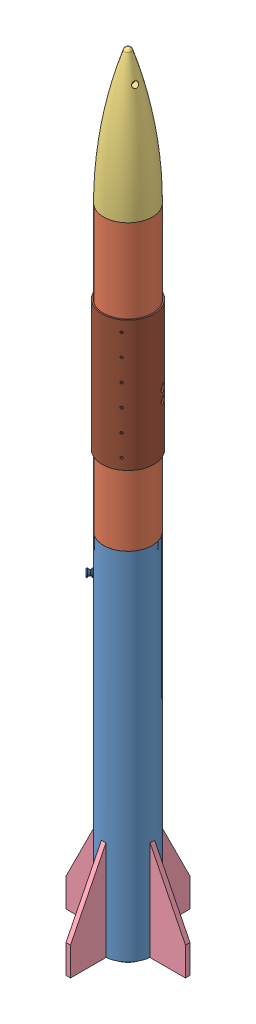
SolidWorks assembly ASSY_ROCKET_MASTER, configuration Default. Lengths in mm. (continued)
Components (placement in the parent): (continued)
- ASSY_HYDRA_MASTER-1: ASSY_HYDRA_MASTER [Default] at (0 713.5 0) x (0.707107 0 0.707107) z (0 1 0) size (64 66.9 228.49) (continued)
  - HYDRA_V4_POWER-1: HYDRA_V4_POWER [Default] at (-0.0043 -0.002 -7.6116) size (50.15 44.15 11.77) (continued)
    - D5-1: D5 [Default] at origin size (1.6 1.5 0.55) (continued)
      - 150066xx54050-1: 150066xx54050 [Default] at (20.5 9.5 0) x (0 1 0) z (0 0 1) size (1.5 1.6 0.55) (continued)
        - body_2-1: body_2 [Default] at origin size (1.5 1.6 0.2)
        - Pads-1: Pads [Default] at origin size (1.4 1.6 0.19)
        - Dome-1: Dome [Default] x (0 -1 0) z (0 0 1) size (1.1 1.5 0.36)
    - D1-1: D1 [Default] at origin size (1.6 1.5 0.55)
      - 150066xx54050-1: 150066xx54050 [Default] at (19 12.5 0) x (0 1 0) z (0 0 1) size (1.5 1.6 0.55)
        - body_2-1: body_2 [Default] at origin size (1.5 1.6 0.2)
        - Pads-1: Pads [Default] at origin size (1.4 1.6 0.19)
        - Dome-1: Dome [Default] x (0 -1 0) z (0 0 1) size (1.1 1.5 0.36)
    - U14-1: U14 [Default] at origin size (4.5 6.6 1.15)
      - 7393011952-1: 7393011952 [Default] at (-9 -10.5 -2.8116) size (4.5 6.6 1.15)
        - Extruded_2-1: Extruded_2 [Default] at origin size (4.5 6.6 1.15)
    - D4-1: D4 [Default] at origin size (1.6 1.5 0.55)
      - 150066xx54050-1: 150066xx54050 [Default] at (14 18.5 0) x (0 1 0) z (0 0 1) size (1.5 1.6 0.55)
        - body_2-1: body_2 [Default] at origin size (1.5 1.6 0.2)
        - Pads-1: Pads [Default] at origin size (1.4 1.6 0.19)
        - Dome-1: Dome [Default] x (0 -1 0) z (0 0 1) size (1.1 1.5 0.36)
    - U13_LS_1-1: U13_LS_1 [Default] at origin size (2.02 2.02 1.01)
      - IC_Texas_Instruments_LM73100RPWR_eec-1: IC_Texas_Instruments_LM73100RPWR_eec [Default] at (-14 2.5 0) x (0 -1 0) z (0 0 1) size (2.02 2.02 1.01)
        - 1_5-1: 1_5 [Default] at origin size (2 2 0.1)
        - 2_6-1: 2_6 [Default] at origin size (2.02 2.02 0.99)
        - Texas Logo Yury-1: Texas Logo Yury [Default] at (-0.3638 0.8313 0.901) x (0 -1 0) z (0 0 1) size (0.26 0.26 0.1)
        - Texas Logo Yury - Copy-1: Texas Logo Yury - Copy [Default] at (-0.335 0.8488 0.901) x (0 -1 0) z (0 0 1) size (0.92 0.24 0.1)
    - U13_LS_0-1: U13_LS_0 [Default] at origin size (2.02 2.02 1.01)
      - IC_Texas_Instruments_LM73100RPWR_eec-1: IC_Texas_Instruments_LM73100RPWR_eec [Default] at (-14 6 0) x (0 -1 0) z (0 0 1) size (2.02 2.02 1.01)
        - 1_5-1: 1_5 [Default] at origin size (2 2 0.1)
        - 2_6-1: 2_6 [Default] at origin size (2.02 2.02 0.99)
        - Texas Logo Yury-1: Texas Logo Yury [Default] at (-0.3638 0.8313 0.901) x (0 -1 0) z (0 0 1) size (0.26 0.26 0.1)
        - Texas Logo Yury - Copy-1: Texas Logo Yury - Copy [Default] at (-0.335 0.8488 0.901) x (0 -1 0) z (0 0 1) size (0.92 0.24 0.1)
    - Y1-1: Y1 [Default] at origin size (3.23 2.53 1.01)
      - Crys_Abracon_ABM8G-12_288MHZ-18-D2Y-T3_eec-1: Crys_Abracon_ABM8G-12_288MHZ-18-D2Y-T3_eec [Default] at (7 20.5 0) x (1 0 0) z (0 0 1) size (3.23 2.53 1.01)
        - body_3-1: body_3 [Default] at origin size (3.23 2.53 1.01)
        - Termination-1: Termination [Default] at origin size (3.2 2.5 0)
        - Marking-1: Marking [Default] at (0 0 1) size (0.25 0.25 0.01)
        - Logo-1: Logo [Default] at (0 0 1) size (1.21 0.73 0.02)
    - U13_LS_2-1: U13_LS_2 [Default] at origin size (2.02 2.02 1.01)
      - IC_Texas_Instruments_LM73100RPWR_eec-1: IC_Texas_Instruments_LM73100RPWR_eec [Default] at (-14 -1 0) x (0 -1 0) z (0 0 1) size (2.02 2.02 1.01)
        - 1_5-1: 1_5 [Default] at origin size (2 2 0.1)
        - 2_6-1: 2_6 [Default] at origin size (2.02 2.02 0.99)
        - Texas Logo Yury-1: Texas Logo Yury [Default] at (-0.3638 0.8313 0.901) x (0 -1 0) z (0 0 1) size (0.26 0.26 0.1)
        - Texas Logo Yury - Copy-1: Texas Logo Yury - Copy [Default] at (-0.335 0.8488 0.901) x (0 -1 0) z (0 0 1) size (0.92 0.24 0.1)
    - U11-1: U11 [Default] at origin size (5.27 5.18 1.1)
      - 6442720976-1: 6442720976 [Default] at (-17.698 12.4027 -1.6116) x (-0.601815 -0.798635 0) z (0 0 -1) size (3.35 4.3 1.1)
    - U10-1: U10 [Default] at origin size (3.99 3.96 1.46)
      - IC_Texas_Instruments_TLV3502AIDCNT_eec-1: IC_Texas_Instruments_TLV3502AIDCNT_eec [Default] at (-18.5 -12.5 0) x (-0.573576 0.819152 0) z (0 0 1) size (2.8 2.9 1.46)
        - IC_BODY-1: IC_BODY [Default] at (0 0 0.15) size (1.6 2.9 1.31)
        - IC_LEG-1: IC_LEG [Default] at (-1.4 1.1375 0) x (1 0 0) z (0 -1 0) size (0.6 0.86 0.3)
        - IC_LEG-2: IC_LEG [Default] at (-1.4 0.4875 0) x (1 0 0) z (0 -1 0) size (0.6 0.86 0.3)
        - IC_LEG-3: IC_LEG [Default] at (-1.4 -0.1625 0) x (1 0 0) z (0 -1 0) size (0.6 0.86 0.3)
        - IC_LEG-4: IC_LEG [Default] at (-1.4 -0.8125 0) x (1 0 0) z (0 -1 0) size (0.6 0.86 0.3)
        - circle-1: circle [Default] at (-0.3239 0.9759 1.451) x (1 0 0) z (0 0 -1) size (0.4 0.4 0.01)
        - Texas Instruments-1: Texas Instruments [Default] at (0.5881 -1.1329 1.45) size (1.22 0.29 0.01)
        - IC_LEG_MIR3-1: IC_LEG_MIR3 [Default] at (1.4 1.1375 0) x (-1 0 0) z (0 1 0) size (0.6 0.86 0.3)
        - IC_LEG_MIR3-2: IC_LEG_MIR3 [Default] at (1.4 0.4875 0) x (-1 0 0) z (0 1 0) size (0.6 0.86 0.3)
        - IC_LEG_MIR3-3: IC_LEG_MIR3 [Default] at (1.4 -0.1625 0) x (-1 0 0) z (0 1 0) size (0.6 0.86 0.3)
        - IC_LEG_MIR3-4: IC_LEG_MIR3 [Default] at (1.4 -0.8125 0) x (-1 0 0) z (0 1 0) size (0.6 0.86 0.3)
    - U9-1: U9 [Default] at origin size (11.99 11.99 1.61)
      - 6684174704-1: 6684174704 [Default] at (-3 16.5 0) x (-1 0 0) z (0 0 1) size (11.99 11.99 1.61)
    - U7-1: U7 [Default] at origin size (3 3 1)
      - 7389152896-1: 7389152896 [Default] at (-0.5 1 0) size (3 3 1)
        - Extruded_4-1: Extruded_4 [Default] at origin size (3 3 1)
    - U6-1: U6 [Default] at origin size (3 3 1)
      - 7389152896-1: 7389152896 [Default] at (-0.5 5.5 0) size (3 3 1)
        - Extruded_4-1: Extruded_4 [Default] at origin size (3 3 1)
    - SW3-1: SW3 [Default] at origin size (2.53 3.5 1.01)
      - Switch_C&K_Components_KXT331LHS_eec-1: Switch_C&K_Components_KXT331LHS_eec [Default] at (-13.5 17.5 0) x (0 1 0) z (0 0 1) size (3.5 2.53 1.01)
        - terminals_3-1: terminals_3 [Default] at origin size (3.5 1.3 0.06)
        - body_3-1: body_3 [Default] at origin size (3.23 2.53 1.01)
        - button top-1: button top [Default] at (0 0 0.385) size (3.2 2.2 0.32)
        - logo_3-1: logo_3 [Default] at (0 0 0.41) size (0.93 0.46 0.01)
    - L2-1: L2 [Default] at origin size (3.65 3.01 2.02)
      - Ind_Vishay_IHLP1212BZER2R2M11_eec-1: Ind_Vishay_IHLP1212BZER2R2M11_eec [Default] at (-5.5 1 0) x (-1 0 0) z (0 0 1) size (3.65 3.01 2.02)
        - body_5-1: body_5 [Default] at origin size (3 3.01 2.01)
        - Pins_2-1: Pins_2 [Default] at origin size (3.65 0.5 1.6)
        - Logo_2-1: Logo_2 [Default] at (0 0 2) size (0.48 0.18 0.02)
    - L1-1: L1 [Default] at origin size (3.65 3.01 2.02)
      - Ind_Vishay_IHLP1212BZER2R2M11_eec-1: Ind_Vishay_IHLP1212BZER2R2M11_eec [Default] at (-5.5 5.5 0) x (-1 0 0) z (0 0 1) size (3.65 3.01 2.02)
        - body_5-1: body_5 [Default] at origin size (3 3.01 2.01)
        - Pins_2-1: Pins_2 [Default] at origin size (3.65 0.5 1.6)
        - Logo_2-1: Logo_2 [Default] at (0 0 2) size (0.48 0.18 0.02)
    - J6-1: J6 [Default] at origin size (10.53 10.1 7.35)
      - FTSH-105-01-F-D-RA-K-1: FTSH-105-01-F-D-RA-K [Default] at (-15.9584 11.7222 2.5) x (-0.601815 -0.798636 0) z (0 0 -1) size (6.27 8.46 7.35)
        - FTSH-105-01-F-D-RA-K_body-1: FTSH-105-01-F-D-RA-K_body [Default] at origin size (6.27 5.71 5.08)
        - FTSH-105-01-F-D-RA-K_pins1-1: FTSH-105-01-F-D-RA-K_pins1 [Default] at origin size (5.49 4.29 1.68)
        - FTSH-105-01-F-D-RA-K_pins2-1: FTSH-105-01-F-D-RA-K_pins2 [Default] at origin size (5.49 3.5 5.65)
    - D3-1: D3 [Default] at origin size (1.6 1.5 0.55)
      - 150066xx54050-1: 150066xx54050 [Default] at (17 15.5 0) x (0 1 0) z (0 0 1) size (1.5 1.6 0.55)
        - body_2-1: body_2 [Default] at origin size (1.5 1.6 0.2)
        - Pads-1: Pads [Default] at origin size (1.4 1.6 0.19)
        - Dome-1: Dome [Default] x (0 -1 0) z (0 0 1) size (1.1 1.5 0.36)
    - C14-1: C14 [Default] at origin size (3.01 3 2.01)
      - Cap_Taiyo_Yuden_EMK212BBJ226MG-T_eec-1: Cap_Taiyo_Yuden_EMK212BBJ226MG-T_eec [Default] at (-11 1 0) x (0 1 0) z (0 0 1) size (3 3.01 2.01)
        - terminals_5-1: terminals_5 [Default] at origin size (2.01 1.26 1.46)
        - body_5-1: body_5 [Default] at origin size (3 3.01 2.01)
        - logo_5-1: logo_5 [Default] at (0.1719 0.8617 1.45) size (0.67 0.05 0)
    - C10-1: C10 [Default] at origin size (3.01 3 2.01)
      - Cap_Taiyo_Yuden_EMK212BBJ226MG-T_eec-1: Cap_Taiyo_Yuden_EMK212BBJ226MG-T_eec [Default] at (2.5 5 -1.6116) x (0 -1 0) z (0 0 -1) size (3 3.01 2.01)
        - terminals_5-1: terminals_5 [Default] at origin size (2.01 1.26 1.46)
        - body_5-1: body_5 [Default] at origin size (3 3.01 2.01)
        - logo_5-1: logo_5 [Default] at (0.1719 0.8617 1.45) size (0.67 0.05 0)
    - C9-1: C9 [Default] at origin size (3.01 3 2.01)
      - Cap_Taiyo_Yuden_EMK212BBJ226MG-T_eec-1: Cap_Taiyo_Yuden_EMK212BBJ226MG-T_eec [Default] at (-11 5.5 0) x (0 1 0) z (0 0 1) size (3 3.01 2.01)
        - terminals_5-1: terminals_5 [Default] at origin size (2.01 1.26 1.46)
        - body_5-1: body_5 [Default] at origin size (3 3.01 2.01)
        - logo_5-1: logo_5 [Default] at (0.1719 0.8617 1.45) size (0.67 0.05 0)
    - C8-1: C8 [Default] at origin size (1.26 2.01 1.46)
      - Cap_Murata_GRM21BC71C106KE11L_eec-1: Cap_Murata_GRM21BC71C106KE11L_eec [Default] at (-9 5.5 0) x (0 1 0) z (0 0 1) size (2.01 1.26 1.46)
        - body_6-1: body_6 [Default] x (-1 0 0) z (0 0 1) size (1.1 1.25 1.45)
        - side-1: side [Default] at (-0.7 0.2667 0) x (-1 0 0) z (0 0 1) size (0.46 1.26 1.46)
        - side-2: side [Default] at (0.7 0.2667 1.45) x (1 0 0) z (0 0 -1) size (0.46 1.26 1.46)
        - Murata_2-1: Murata_2 [Default] at (-0.7353 -0.8898 1.447) size (0.62 0.15 0.01)
    - J3-1: J3 [Default] at origin size (13.3 13.95 7)
      - 6684174944-1: 6684174944 [Default] at (-9 -13 0) x (-1 0 0) z (0 1 0) size (13.3 7 13.95)
    - J5-1: J5 [Default] at origin size (5.84 15.88 6.73)
      - TFML-110-02-S-D-A-1: TFML-110-02-S-D-A [Default] at (20 0 0) x (0 1 0) z (1 0 0) size (15.88 6.73 5.84)
        - TFML-110-02-L-D-A_terminal-1: TFML-110-02-L-D-A_terminal [Default] at origin size (15.88 6.73 5.72)
        - TFML-110-02-L-D-L_pins-1: TFML-110-02-L-D-L_pins [Default] at origin size (12.7 4.01 1.78)
        - TFML-110-02-L-D-S-2_pins-1: TFML-110-02-L-D-S-2_pins [Default] at origin size (12.7 0.83 5.84)
    - J4-1: J4 [Default] at origin size (5.84 15.88 6.73)
      - TFML-110-02-S-D-A-1: TFML-110-02-S-D-A [Default] at (-20 0 0) x (0 1 0) z (1 0 0) size (15.88 6.73 5.84)
        - TFML-110-02-L-D-A_terminal-1: TFML-110-02-L-D-A_terminal [Default] at origin size (15.88 6.73 5.72)
        - TFML-110-02-L-D-L_pins-1: TFML-110-02-L-D-L_pins [Default] at origin size (12.7 4.01 1.78)
        - TFML-110-02-L-D-S-2_pins-1: TFML-110-02-L-D-S-2_pins [Default] at origin size (12.7 0.83 5.84)
    - J2-1: J2 [Default] at origin size (4.2 15.88 5.84)
      - SFML-110-02-L-D-A-1: SFML-110-02-L-D-A [Default] at (20 0 -1.6116) x (0 -1 0) z (1 0 0) size (15.88 5.84 4.2)
        - SFML-110-02-L-D-A_terminal-1: SFML-110-02-L-D-A_terminal [Default] at origin size (15.88 5.84 3.68)
        - C-10-02-D-L_pins-1: C-10-02-D-L_pins [Default] at origin size (12.7 1.18 4.09)
    - J1-1: J1 [Default] at origin size (4.2 15.88 5.84)
      - SFML-110-02-L-D-A-1: SFML-110-02-L-D-A [Default] at (-20 0 -1.6116) x (0 -1 0) z (1 0 0) size (15.88 5.84 4.2)
        - SFML-110-02-L-D-A_terminal-1: SFML-110-02-L-D-A_terminal [Default] at origin size (15.88 5.84 3.68)
        - C-10-02-D-L_pins-1: C-10-02-D-L_pins [Default] at origin size (12.7 1.18 4.09)
    - SW1-1: SW1 [Default] at origin size (2.53 3.5 1.01)
      - Switch_C&K_Components_KXT331LHS_eec-1: Switch_C&K_Components_KXT331LHS_eec [Default] at (10.5 19.5 0) x (0 -1 0) z (0 0 1) size (3.5 2.53 1.01)
        - terminals_3-1: terminals_3 [Default] at origin size (3.5 1.3 0.06)
        - body_3-1: body_3 [Default] at origin size (3.23 2.53 1.01)
        - button top-1: button top [Default] at (0 0 0.385) size (3.2 2.2 0.32)
        - logo_3-1: logo_3 [Default] at (0 0 0.41) size (0.93 0.46 0.01)
  - HYDRA_V4_POWER-2: HYDRA_V4_POWER [Default] at (-0.0043 -0.002 -15.2232) size (50.15 44.15 11.77)
    - Board-1: Board [Default] at origin size (50.15 44.15 1.61)
      - Open CASCADE STEP translator 7.5 2754.1.1-1: Open CASCADE STEP translator 7.5 2754.1.1 [Default] at (0 0 -1.6116) size (50.15 44.15 1.61)
    - J8-1: J8 [Default] at origin size (8.25 4.85 4.36)
      - Conn_JST_SM04B-GHS-TB_LF_SN_eec-1: Conn_JST_SM04B-GHS-TB_LF_SN_eec [Default] at (6.125 -14.4749 0.1) x (1 0 0) z (0 -1 0) size (8.25 4.36 4.85)
        - body-1: body [Default] at origin size (8.25 4.25 4.05)
        - Pins-1: Pins [Default] at origin size (7.65 2.05 4.85)
        - New Marking-1: New Marking [Default] at (-5.7821 4.251 3.7193) x (1 0 0) z (0 -1 0) size (0.46 0.67 0)
        - JST Logo-1: JST Logo [Default] at (14.4297 4.25 10.8095) x (1 0 0) z (0 1 0) size (1.76 0.68 0.01)
    - J7-1: J7 [Default] at origin size (9.7 4.86 4.36)
      - Conn_JST_SM05B-GHS-TB_LF_SN_eec-1: Conn_JST_SM05B-GHS-TB_LF_SN_eec [Default] at (11.5 -16.5 0) size (9.7 4.86 4.36)
        - 1-1: 1 [Default] at (4.75 2.025 0.1) x (1 0 0) z (0 -1 0) size (9.7 4.36 4.86)
          - 1_2-1: 1_2 [Default] at origin size (5.2 1.05 4.44)
          - SM05B-GHS-TB-1: SM05B-GHS-TB [Default] at origin size (9.7 4.26 4.06)
          - 2_2-1: 2_2 [Default] at origin size (8.9 2.05 2.2)
        - JST Logo adjustable-1: JST Logo adjustable [Default] at (-0.5885 2.016 5.7361) x (-1 0 0) z (0 1 0) size (0.68 0.81 0.01)
    - D5-1: D5 [Default] at origin size (1.6 1.5 0.55)
      - 150066xx54050-1: 150066xx54050 [Default] at (20.5 9.5 0) x (0 1 0) z (0 0 1) size (1.5 1.6 0.55)
        - body_2-1: body_2 [Default] at origin size (1.5 1.6 0.2)
        - Pads-1: Pads [Default] at origin size (1.4 1.6 0.19)
        - Dome-1: Dome [Default] x (0 -1 0) z (0 0 1) size (1.1 1.5 0.36)
    - D1-1: D1 [Default] at origin size (1.6 1.5 0.55)
      - 150066xx54050-1: 150066xx54050 [Default] at (19 12.5 0) x (0 1 0) z (0 0 1) size (1.5 1.6 0.55)
        - body_2-1: body_2 [Default] at origin size (1.5 1.6 0.2)
        - Pads-1: Pads [Default] at origin size (1.4 1.6 0.19)
        - Dome-1: Dome [Default] x (0 -1 0) z (0 0 1) size (1.1 1.5 0.36)
    - U14-1: U14 [Default] at origin size (4.5 6.6 1.15)
      - 7393011952-1: 7393011952 [Default] at (-9 -10.5 -2.8116) size (4.5 6.6 1.15)
        - Extruded_2-1: Extruded_2 [Default] at origin size (4.5 6.6 1.15)
    - D4-1: D4 [Default] at origin size (1.6 1.5 0.55)
      - 150066xx54050-1: 150066xx54050 [Default] at (14 18.5 0) x (0 1 0) z (0 0 1) size (1.5 1.6 0.55)
        - body_2-1: body_2 [Default] at origin size (1.5 1.6 0.2)
        - Pads-1: Pads [Default] at origin size (1.4 1.6 0.19)
        - Dome-1: Dome [Default] x (0 -1 0) z (0 0 1) size (1.1 1.5 0.36)
    - U13_LS_1-1: U13_LS_1 [Default] at origin size (2.02 2.02 1.01)
      - IC_Texas_Instruments_LM73100RPWR_eec-1: IC_Texas_Instruments_LM73100RPWR_eec [Default] at (-14 2.5 0) x (0 -1 0) z (0 0 1) size (2.02 2.02 1.01)
        - 1_5-1: 1_5 [Default] at origin size (2 2 0.1)
        - 2_6-1: 2_6 [Default] at origin size (2.02 2.02 0.99)
        - Texas Logo Yury-1: Texas Logo Yury [Default] at (-0.3638 0.8313 0.901) x (0 -1 0) z (0 0 1) size (0.26 0.26 0.1)
        - Texas Logo Yury - Copy-1: Texas Logo Yury - Copy [Default] at (-0.335 0.8488 0.901) x (0 -1 0) z (0 0 1) size (0.92 0.24 0.1)
    - U13_LS_0-1: U13_LS_0 [Default] at origin size (2.02 2.02 1.01)
      - IC_Texas_Instruments_LM73100RPWR_eec-1: IC_Texas_Instruments_LM73100RPWR_eec [Default] at (-14 6 0) x (0 -1 0) z (0 0 1) size (2.02 2.02 1.01)
        - 1_5-1: 1_5 [Default] at origin size (2 2 0.1)
        - 2_6-1: 2_6 [Default] at origin size (2.02 2.02 0.99)
        - Texas Logo Yury-1: Texas Logo Yury [Default] at (-0.3638 0.8313 0.901) x (0 -1 0) z (0 0 1) size (0.26 0.26 0.1)
        - Texas Logo Yury - Copy-1: Texas Logo Yury - Copy [Default] at (-0.335 0.8488 0.901) x (0 -1 0) z (0 0 1) size (0.92 0.24 0.1)
    - Y1-1: Y1 [Default] at origin size (3.23 2.53 1.01)
      - Crys_Abracon_ABM8G-12_288MHZ-18-D2Y-T3_eec-1: Crys_Abracon_ABM8G-12_288MHZ-18-D2Y-T3_eec [Default] at (7 20.5 0) x (1 0 0) z (0 0 1) size (3.23 2.53 1.01)
        - body_3-1: body_3 [Default] at origin size (3.23 2.53 1.01)
        - Termination-1: Termination [Default] at origin size (3.2 2.5 0)
        - Marking-1: Marking [Default] at (0 0 1) size (0.25 0.25 0.01)
        - Logo-1: Logo [Default] at (0 0 1) size (1.21 0.73 0.02)
    - U13_LS_2-1: U13_LS_2 [Default] at origin size (2.02 2.02 1.01)
      - IC_Texas_Instruments_LM73100RPWR_eec-1: IC_Texas_Instruments_LM73100RPWR_eec [Default] at (-14 -1 0) x (0 -1 0) z (0 0 1) size (2.02 2.02 1.01)
        - 1_5-1: 1_5 [Default] at origin size (2 2 0.1)
        - 2_6-1: 2_6 [Default] at origin size (2.02 2.02 0.99)
        - Texas Logo Yury-1: Texas Logo Yury [Default] at (-0.3638 0.8313 0.901) x (0 -1 0) z (0 0 1) size (0.26 0.26 0.1)
        - Texas Logo Yury - Copy-1: Texas Logo Yury - Copy [Default] at (-0.335 0.8488 0.901) x (0 -1 0) z (0 0 1) size (0.92 0.24 0.1)
    - U11-1: U11 [Default] at origin size (5.27 5.18 1.1)
      - 6442720976-1: 6442720976 [Default] at (-17.698 12.4027 -1.6116) x (-0.601815 -0.798635 0) z (0 0 -1) size (3.35 4.3 1.1)
    - U10-1: U10 [Default] at origin size (3.99 3.96 1.46)
      - IC_Texas_Instruments_TLV3502AIDCNT_eec-1: IC_Texas_Instruments_TLV3502AIDCNT_eec [Default] at (-18.5 -12.5 0) x (-0.573576 0.819152 0) z (0 0 1) size (2.8 2.9 1.46)
        - IC_BODY-1: IC_BODY [Default] at (0 0 0.15) size (1.6 2.9 1.31)
        - IC_LEG-1: IC_LEG [Default] at (-1.4 1.1375 0) x (1 0 0) z (0 -1 0) size (0.6 0.86 0.3)
        - IC_LEG-2: IC_LEG [Default] at (-1.4 0.4875 0) x (1 0 0) z (0 -1 0) size (0.6 0.86 0.3)
        - IC_LEG-3: IC_LEG [Default] at (-1.4 -0.1625 0) x (1 0 0) z (0 -1 0) size (0.6 0.86 0.3)
        - IC_LEG-4: IC_LEG [Default] at (-1.4 -0.8125 0) x (1 0 0) z (0 -1 0) size (0.6 0.86 0.3)
        - circle-1: circle [Default] at (-0.3239 0.9759 1.451) x (1 0 0) z (0 0 -1) size (0.4 0.4 0.01)
        - Texas Instruments-1: Texas Instruments [Default] at (0.5881 -1.1329 1.45) size (1.22 0.29 0.01)
        - IC_LEG_MIR3-1: IC_LEG_MIR3 [Default] at (1.4 1.1375 0) x (-1 0 0) z (0 1 0) size (0.6 0.86 0.3)
        - IC_LEG_MIR3-2: IC_LEG_MIR3 [Default] at (1.4 0.4875 0) x (-1 0 0) z (0 1 0) size (0.6 0.86 0.3)
        - IC_LEG_MIR3-3: IC_LEG_MIR3 [Default] at (1.4 -0.1625 0) x (-1 0 0) z (0 1 0) size (0.6 0.86 0.3)
        - IC_LEG_MIR3-4: IC_LEG_MIR3 [Default] at (1.4 -0.8125 0) x (-1 0 0) z (0 1 0) size (0.6 0.86 0.3)
    - U9-1: U9 [Default] at origin size (11.99 11.99 1.61)
      - 6684174704-1: 6684174704 [Default] at (-3 16.5 0) x (-1 0 0) z (0 0 1) size (11.99 11.99 1.61)
    - U7-1: U7 [Default] at origin size (3 3 1)
      - 7389152896-1: 7389152896 [Default] at (-0.5 1 0) size (3 3 1)
        - Extruded_4-1: Extruded_4 [Default] at origin size (3 3 1)
    - U6-1: U6 [Default] at origin size (3 3 1)
      - 7389152896-1: 7389152896 [Default] at (-0.5 5.5 0) size (3 3 1)
        - Extruded_4-1: Extruded_4 [Default] at origin size (3 3 1)
    - SW3-1: SW3 [Default] at origin size (2.53 3.5 1.01)
      - Switch_C&K_Components_KXT331LHS_eec-1: Switch_C&K_Components_KXT331LHS_eec [Default] at (-13.5 17.5 0) x (0 1 0) z (0 0 1) size (3.5 2.53 1.01)
        - terminals_3-1: terminals_3 [Default] at origin size (3.5 1.3 0.06)
        - body_3-1: body_3 [Default] at origin size (3.23 2.53 1.01)
        - button top-1: button top [Default] at (0 0 0.385) size (3.2 2.2 0.32)
        - logo_3-1: logo_3 [Default] at (0 0 0.41) size (0.93 0.46 0.01)
    - L2-1: L2 [Default] at origin size (3.65 3.01 2.02)
      - Ind_Vishay_IHLP1212BZER2R2M11_eec-1: Ind_Vishay_IHLP1212BZER2R2M11_eec [Default] at (-5.5 1 0) x (-1 0 0) z (0 0 1) size (3.65 3.01 2.02)
        - body_5-1: body_5 [Default] at origin size (3 3.01 2.01)
        - Pins_2-1: Pins_2 [Default] at origin size (3.65 0.5 1.6)
        - Logo_2-1: Logo_2 [Default] at (0 0 2) size (0.48 0.18 0.02)
    - L1-1: L1 [Default] at origin size (3.65 3.01 2.02)
      - Ind_Vishay_IHLP1212BZER2R2M11_eec-1: Ind_Vishay_IHLP1212BZER2R2M11_eec [Default] at (-5.5 5.5 0) x (-1 0 0) z (0 0 1) size (3.65 3.01 2.02)
        - body_5-1: body_5 [Default] at origin size (3 3.01 2.01)
        - Pins_2-1: Pins_2 [Default] at origin size (3.65 0.5 1.6)
        - Logo_2-1: Logo_2 [Default] at (0 0 2) size (0.48 0.18 0.02)
    - J6-1: J6 [Default] at origin size (10.53 10.1 7.35)
      - FTSH-105-01-F-D-RA-K-1: FTSH-105-01-F-D-RA-K [Default] at (-15.9584 11.7222 2.5) x (-0.601815 -0.798636 0) z (0 0 -1) size (6.27 8.46 7.35)
        - FTSH-105-01-F-D-RA-K_body-1: FTSH-105-01-F-D-RA-K_body [Default] at origin size (6.27 5.71 5.08)
        - FTSH-105-01-F-D-RA-K_pins1-1: FTSH-105-01-F-D-RA-K_pins1 [Default] at origin size (5.49 4.29 1.68)
        - FTSH-105-01-F-D-RA-K_pins2-1: FTSH-105-01-F-D-RA-K_pins2 [Default] at origin size (5.49 3.5 5.65)
    - D3-1: D3 [Default] at origin size (1.6 1.5 0.55)
      - 150066xx54050-1: 150066xx54050 [Default] at (17 15.5 0) x (0 1 0) z (0 0 1) size (1.5 1.6 0.55)
        - body_2-1: body_2 [Default] at origin size (1.5 1.6 0.2)
        - Pads-1: Pads [Default] at origin size (1.4 1.6 0.19)
        - Dome-1: Dome [Default] x (0 -1 0) z (0 0 1) size (1.1 1.5 0.36)
    - C14-1: C14 [Default] at origin size (3.01 3 2.01)
      - Cap_Taiyo_Yuden_EMK212BBJ226MG-T_eec-1: Cap_Taiyo_Yuden_EMK212BBJ226MG-T_eec [Default] at (-11 1 0) x (0 1 0) z (0 0 1) size (3 3.01 2.01)
        - terminals_5-1: terminals_5 [Default] at origin size (2.01 1.26 1.46)
        - body_5-1: body_5 [Default] at origin size (3 3.01 2.01)
        - logo_5-1: logo_5 [Default] at (0.1719 0.8617 1.45) size (0.67 0.05 0)
    - C10-1: C10 [Default] at origin size (3.01 3 2.01)
      - Cap_Taiyo_Yuden_EMK212BBJ226MG-T_eec-1: Cap_Taiyo_Yuden_EMK212BBJ226MG-T_eec [Default] at (2.5 5 -1.6116) x (0 -1 0) z (0 0 -1) size (3 3.01 2.01)
        - terminals_5-1: terminals_5 [Default] at origin size (2.01 1.26 1.46)
        - body_5-1: body_5 [Default] at origin size (3 3.01 2.01)
        - logo_5-1: logo_5 [Default] at (0.1719 0.8617 1.45) size (0.67 0.05 0)
    - C9-1: C9 [Default] at origin size (3.01 3 2.01)
      - Cap_Taiyo_Yuden_EMK212BBJ226MG-T_eec-1: Cap_Taiyo_Yuden_EMK212BBJ226MG-T_eec [Default] at (-11 5.5 0) x (0 1 0) z (0 0 1) size (3 3.01 2.01)
        - terminals_5-1: terminals_5 [Default] at origin size (2.01 1.26 1.46)
        - body_5-1: body_5 [Default] at origin size (3 3.01 2.01)
        - logo_5-1: logo_5 [Default] at (0.1719 0.8617 1.45) size (0.67 0.05 0)
    - C8-1: C8 [Default] at origin size (1.26 2.01 1.46)
      - Cap_Murata_GRM21BC71C106KE11L_eec-1: Cap_Murata_GRM21BC71C106KE11L_eec [Default] at (-9 5.5 0) x (0 1 0) z (0 0 1) size (2.01 1.26 1.46)
        - body_6-1: body_6 [Default] x (-1 0 0) z (0 0 1) size (1.1 1.25 1.45)
        - side-1: side [Default] at (-0.7 0.2667 0) x (-1 0 0) z (0 0 1) size (0.46 1.26 1.46)
        - side-2: side [Default] at (0.7 0.2667 1.45) x (1 0 0) z (0 0 -1) size (0.46 1.26 1.46)
        - Murata_2-1: Murata_2 [Default] at (-0.7353 -0.8898 1.447) size (0.62 0.15 0.01)
    - J3-1: J3 [Default] at origin size (13.3 13.95 7)
      - 6684174944-1: 6684174944 [Default] at (-9 -13 0) x (-1 0 0) z (0 1 0) size (13.3 7 13.95)
    - J5-1: J5 [Default] at origin size (5.84 15.88 6.73)
      - TFML-110-02-S-D-A-1: TFML-110-02-S-D-A [Default] at (20 0 0) x (0 1 0) z (1 0 0) size (15.88 6.73 5.84)
        - TFML-110-02-L-D-A_terminal-1: TFML-110-02-L-D-A_terminal [Default] at origin size (15.88 6.73 5.72)
        - TFML-110-02-L-D-L_pins-1: TFML-110-02-L-D-L_pins [Default] at origin size (12.7 4.01 1.78)
        - TFML-110-02-L-D-S-2_pins-1: TFML-110-02-L-D-S-2_pins [Default] at origin size (12.7 0.83 5.84)
    - J4-1: J4 [Default] at origin size (5.84 15.88 6.73)
      - TFML-110-02-S-D-A-1: TFML-110-02-S-D-A [Default] at (-20 0 0) x (0 1 0) z (1 0 0) size (15.88 6.73 5.84)
        - TFML-110-02-L-D-A_terminal-1: TFML-110-02-L-D-A_terminal [Default] at origin size (15.88 6.73 5.72)
        - TFML-110-02-L-D-L_pins-1: TFML-110-02-L-D-L_pins [Default] at origin size (12.7 4.01 1.78)
        - TFML-110-02-L-D-S-2_pins-1: TFML-110-02-L-D-S-2_pins [Default] at origin size (12.7 0.83 5.84)
    - J2-1: J2 [Default] at origin size (4.2 15.88 5.84)
      - SFML-110-02-L-D-A-1: SFML-110-02-L-D-A [Default] at (20 0 -1.6116) x (0 -1 0) z (1 0 0) size (15.88 5.84 4.2)
        - SFML-110-02-L-D-A_terminal-1: SFML-110-02-L-D-A_terminal [Default] at origin size (15.88 5.84 3.68)
        - C-10-02-D-L_pins-1: C-10-02-D-L_pins [Default] at origin size (12.7 1.18 4.09)
    - J1-1: J1 [Default] at origin size (4.2 15.88 5.84)
      - SFML-110-02-L-D-A-1: SFML-110-02-L-D-A [Default] at (-20 0 -1.6116) x (0 -1 0) z (1 0 0) size (15.88 5.84 4.2)
        - SFML-110-02-L-D-A_terminal-1: SFML-110-02-L-D-A_terminal [Default] at origin size (15.88 5.84 3.68)
        - C-10-02-D-L_pins-1: C-10-02-D-L_pins [Default] at origin size (12.7 1.18 4.09)
    - SW1-1: SW1 [Default] at origin size (2.53 3.5 1.01)
      - Switch_C&K_Components_KXT331LHS_eec-1: Switch_C&K_Components_KXT331LHS_eec [Default] at (10.5 19.5 0) x (0 -1 0) z (0 0 1) size (3.5 2.53 1.01)
        - terminals_3-1: terminals_3 [Default] at origin size (3.5 1.3 0.06)
        - body_3-1: body_3 [Default] at origin size (3.23 2.53 1.01)
        - button top-1: button top [Default] at (0 0 0.385) size (3.2 2.2 0.32)
        - logo_3-1: logo_3 [Default] at (0 0 0.41) size (0.93 0.46 0.01)
  - HYDRA_CRADDLE-1: HYDRA_CRADDLE [Default] x (1 0 0) z (0 -1 0) size (64 183 64)
  - HYDRA_PRIMARY_BATTERY-1: HYDRA_PRIMARY_BATTERY [Default] at (0 -1.383 -93.5) x (0 1 0) z (1 0 0) size (32.77 69 25)
  - HYDRA_LORA_MODULE-1: HYDRA_LORA_MODULE [Default] at (16 4.75 -75.5) x (0 1 0) z (0 0 -1) size (24 6.5 55.5)
  - HYDRA_GPS_ANTENNA-1: HYDRA_GPS_ANTENNA [Default] at (16.2218 13.4159 32.2782) x (0.642788 -0.766044 0) z (-0.541675 -0.454519 0.707107) size (18.6 6.8 21.3)
  - HYDRA_STUBBY_433_ANTENNA-1: HYDRA_STUBBY_433_ANTENNA [Default] at (18 -2 -106.5) x (-0.546944 -0.837169 0) z (0.837169 -0.546944 0) size (9.24 43 8)
  - COTS_CAMERA_MODULE-2: COTS_CAMERA_MODULE [Default] at (6.3277 -18.5548 -100) x (-0.939693 -0.34202 0) z (0.34202 -0.939693 0) size (14.2 17.5 14.2)
  - COTS_EYE_BOLT-1: COTS_EYE_BOLT [Default] at (-19.9239 1.7431 43.2) x (1 0 0) z (0 -1 0) size (18.5 38.79 4.5)
  - COTS_EYE_BOLT-2: COTS_EYE_BOLT [Default] at (-19.9239 1.7431 -87.2) x (-0.157845 -0.987464 0) z (0.987464 -0.157845 0) size (18.5 38.79 4.5)
  - COTS_WASHER_3_16-1: COTS_WASHER_3_16 [Default] at (-19.9239 1.7431 60.5) x (1 0 0) z (0 -1 0) size (11.2 0.7 11.2)
  - COTS_WASHER_3_16-2: COTS_WASHER_3_16 [Default] at (-19.9239 1.7431 51.3) x (1 0 0) z (0 -1 0) size (11.2 0.7 11.2)
  - COTS_WASHER_3_16-3: COTS_WASHER_3_16 [Default] at (-19.9239 1.7431 -95.3) x (1 0 0) z (0 1 0) size (11.2 0.7 11.2)
  - COTS_WASHER_3_16-4: COTS_WASHER_3_16 [Default] at (-19.9239 1.7431 -104.5) x (1 0 0) z (0 1 0) size (11.2 0.7 11.2)
  - HYDRA_UMBILICAL_CONNECTOR_8POS-1: HYDRA_UMBILICAL_CONNECTOR_8POS [Default] at (-10.2425 26.3386 -44.52) x (0 0 1) z (-0.362438 0.932008 0) size (34.96 9.2 6)
  - HYDRA_UMBILICAL_COVER-1: HYDRA_UMBILICAL_COVER [Default] at (-12.4135 31.9213 -24.52) x (0.932008 0.362438 0) z (-0.362438 0.932008 0) size (12.23 40.34 3.99)
  - COTS_METAL_M3_STANDOFF-1: COTS_METAL_M3_STANDOFF [Default] at (9 -0.5 55.5) x (-0.5 -0.866025 0) z (-0.866025 0.5 0) size (5.31 14 4.6)
  - COTS_METAL_M3_STANDOFF-2: COTS_METAL_M3_STANDOFF [Default] at (-9 -0.5 55.5) x (-0.5 -0.866025 0) z (-0.866025 0.5 0) size (5.31 14 4.6)
  - COTS_METAL_M3_STANDOFF-3: COTS_METAL_M3_STANDOFF [Default] at (9 -0.5 -99.5) x (0.5 -0.866025 0) z (0.866025 0.5 0) size (5.31 14 4.6)
  - COTS_METAL_M3_STANDOFF-4: COTS_METAL_M3_STANDOFF [Default] at (-9 -0.5 -99.5) x (1 0 0) z (0 1 0) size (5.31 14 4.6)
  - HYDRA_PCB_CLAMP-1: HYDRA_PCB_CLAMP [Default] at (-30.4 -16 -0.8) x (1 0 0) z (0 -1 0) size (9.12 36.4 6)
  - HYDRA_PCB_CLAMP-2: HYDRA_PCB_CLAMP [Default] at (30.4 -16 -0.8) x (-1 0 0) z (0 -1 0) size (9.12 36.4 6)
  - COTS_BARREL_JACK_FOR_RBF-1: COTS_BARREL_JACK_FOR_RBF [Default] at (9.8722 30.4555 -30.6) x (0.329101 -0.118159 0.936873) z (-0.881762 0.316585 0.34967) size (10 12 10)
  - COTS_BARREL_JACK_FOR_RBF-2: COTS_BARREL_JACK_FOR_RBF [Default] at (9.8722 30.4555 -45.8) x (0.911416 -0.327232 -0.249481) z (0.234805 -0.084304 0.96838) size (10 12 10)
  - HYDRA_CAMERA_COVER-1: HYDRA_CAMERA_COVER [Default] at (6.8404 -18.7939 59.5) x (-0.939693 -0.34202 0) z (-0.34202 0.939693 0) size (29.5 9.47 19)
  - HYDRA_CAMERA_COVER-2: HYDRA_CAMERA_COVER [Default] at (6.8404 -18.7939 -103.5) x (0.939693 0.34202 0) z (-0.34202 0.939693 0) size (29.5 9.47 19)
  - COTS_CAMERA_MODULE-3: COTS_CAMERA_MODULE [Default] at (7.3531 -19.0329 56) x (0.939693 0.34202 0) z (0.34202 -0.939693 0) size (14.2 17.5 14.2)
- ROCKET_MOTOR_TUBE-1: ROCKET_MOTOR_TUBE [Default] at (0 -10 0) size (41.6 279.4 41.6)
- ROCKET_CENTERING_RING-1: ROCKET_CENTERING_RING [Default] at (0 3.65 0) size (64.5 6.35 64.5)
- ROCKET_CENTERING_RING-2: ROCKET_CENTERING_RING [Default] at (0 130 0) size (64.5 6.35 64.5)
- ROCKET_CENTERING_RING-3: ROCKET_CENTERING_RING [Default] at (0 260 0) size (64.5 6.35 64.5)
- ROCKET_BAFFLE_TUBE-1: ROCKET_BAFFLE_TUBE [Default] at (0 437.6 0) x (0.999882 0 0.015331) z (0 -1 0) size (64.52 64.52 76.2)
- ROCKET_BAFFLE_PLATE-1: ROCKET_BAFFLE_PLATE [Default] at (0 361.4 0) x (0.999882 0 0.015331) z (-0.015331 0 0.999882) size (63 3 63)
- ROCKET_BAFFLE_PLATE-2: ROCKET_BAFFLE_PLATE [Default] at (0 434.6 0) x (0.999882 0 0.015331) z (-0.015331 0 0.999882) size (63 3 63)
- COTS_WASHER_3_16-1: COTS_WASHER_3_16 [Default] at (0 433.9 0) x (0.997264 0 0.073924) z (-0.073924 0 0.997264) size (11.2 0.7 11.2)
- COTS_WASHER_3_16-3: COTS_WASHER_3_16 [Default] at (0 437.6 0) x (0.997264 0 0.073924) z (-0.073924 0 0.997264) size (11.2 0.7 11.2)
- COTS_EYE_BOLT-3: COTS_EYE_BOLT [Default] at (0 420.3 0) size (18.5 38.79 4.5)
- ROCKET_RAIL_BUTTON-1: ROCKET_RAIL_BUTTON [Default] at (-24.2184 450 24.2184) x (0.515012 0.685219 0.515012) z (0.484523 -0.728337 0.484523) size (9.4 7.62 9.4)
- ROCKET_RAIL_BUTTON-2: ROCKET_RAIL_BUTTON [Default] at (-24.2184 25 24.2184) x (-0.068335 0.995319 -0.068335) z (0.703797 0.09664 0.703797) size (9.4 7.62 9.4)
- JIG_HYDRA_CRADDLE_HOLES-1: JIG_HYDRA_CRADDLE_HOLES [Default] at (0 783 0) x (0.707107 0 0.707107) z (0.707107 0 -0.707107) size (73 183 73)
Mates (geometry in assembly coordinates):
- Coincident1: coincident anti-aligned: plane of ROCKET_BODY_TUBE_LOWER-1 through (0 500 0) normal (0 1 0); plane of ROCKET_BODY_TUBE_UPPER-1 through (0 500 0) normal (0 -1 0)
- Concentric1: concentric aligned: cylinder of ROCKET_BODY_TUBE_LOWER-1 through (0 500 0) axis (0 -1 0) radius 34.25; cylinder of ROCKET_BODY_TUBE_UPPER-1 through (0 900 0) axis (0 -1 0) radius 34.25
- Coincident2: coincident anti-aligned: plane of ROCKET_BODY_TUBE_UPPER-1 through (0 900 0) normal (0 1 0); plane of ROCKET_NOSE_CONE-1 through (33.0654 900 8.93) normal (0 -1 0)
- Concentric2: concentric aligned: cylinder of ROCKET_BODY_TUBE_UPPER-1 through (0 900 0) axis (0 -1 0) radius 34.25; circle of ROCKET_NOSE_CONE-1
- Distance1: distance = 90 mm aligned: plane of ROCKET_BODY_COUPLER-1 through (0 590 0) normal (0 1 0); plane of ROCKET_BODY_TUBE_LOWER-1 through (0 500 0) normal (0 1 0)
- Concentric3: concentric aligned: cylinder of ROCKET_BODY_TUBE_LOWER-1 through (0 500 0) axis (0 -1 0) radius 32.5; cylinder of ROCKET_BODY_COUPLER-1 through (0 590 0) axis (0 -1 0) radius 32.45
- Coincident5: coincident aligned: plane of ROCKET_MOTOR_TUBE-1 through (0 -10 0) normal (0 0 1)
- Coincident6: coincident aligned: plane of ROCKET_MOTOR_TUBE-1 through (0 -10 0) normal (1 0 0)
- Distance2: distance = 10 mm: plane of assembly through (0 0 0) normal (0 1 0); plane of assembly; plane of ROCKET_MOTOR_TUBE-1 through (0 -10 0) normal (0 1 0)
- Coincident8: coincident aligned: plane of ROCKET_CENTERING_RING-1 through (0 3.65 0) normal (1 0 0)
- Coincident9: coincident aligned: plane of ROCKET_CENTERING_RING-1 through (0 3.65 0) normal (0 0 1)
- Distance3: distance = 3.65 mm aligned: plane of ROCKET_CENTERING_RING-1 through (0 3.65 0) normal (0 1 0)
- Coincident11: coincident aligned: plane of ROCKET_CENTERING_RING-2 through (0 130 0) normal (0 0 1)
- Coincident12: coincident aligned: plane of ROCKET_CENTERING_RING-2 through (0 130 0) normal (1 0 0)
- Distance4: distance = 130 mm: plane of assembly through (0 0 0) normal (0 1 0); plane of assembly; plane of ROCKET_CENTERING_RING-2 through (0 130 0) normal (0 1 0)
- Coincident14: coincident aligned: plane of ROCKET_CENTERING_RING-3 through (0 260 0) normal (1 0 0)
- Coincident15: coincident aligned: plane of ROCKET_CENTERING_RING-3 through (0 260 0) normal (0 0 1)
- Distance5: distance = 260 mm aligned: plane of ROCKET_CENTERING_RING-3 through (0 260 0) normal (0 1 0)
- Concentric4: concentric anti-aligned: cylinder of ROCKET_BAFFLE_TUBE-1 through (0 361.4 0) axis (0 1 0) radius 31.5; cylinder of ROCKET_BAFFLE_PLATE-1 through (0 364.4 0) axis (0 -1 0) radius 31.5
- Coincident16: coincident aligned: plane of ROCKET_BAFFLE_TUBE-1 through (0 361.4 0) normal (0 -1 0); plane of ROCKET_BAFFLE_PLATE-1 through (0 361.4 0) normal (0 -1 0)
- Concentric5: concentric anti-aligned: cylinder of ROCKET_BAFFLE_TUBE-1 through (0 361.4 0) axis (0 1 0) radius 31.5; cylinder of ROCKET_BAFFLE_PLATE-2 through (0 437.6 0) axis (0 -1 0) radius 31.5
- Coincident17: coincident aligned: plane of ROCKET_BAFFLE_TUBE-1 through (0 437.6 0) normal (0 1 0); plane of ROCKET_BAFFLE_PLATE-2 through (0 437.6 0) normal (0 1 0)
- Concentric6: concentric anti-aligned: cylinder of ROCKET_BODY_TUBE_LOWER-1 through (0 500 0) axis (0 -1 0) radius 32.5; cylinder of ROCKET_BAFFLE_TUBE-1 through (0 361.4 0) axis (0 1 0) radius 32.258
- Coincident18: coincident anti-aligned: plane of ROCKET_BODY_COUPLER-1 through (0 437.6 0) normal (0 -1 0); plane of ROCKET_BAFFLE_TUBE-1 through (0 437.6 0) normal (0 1 0)
- Concentric7: concentric aligned: cylinder of ROCKET_BAFFLE_PLATE-2 through (0 437.6 0) axis (0 -1 0) radius 2.5; cylinder of COTS_WASHER_3_16-1 through (0 434.6 0) axis (0 -1 0) radius 2.7
- Concentric8: concentric aligned: cylinder of ROCKET_BAFFLE_PLATE-2 through (0 437.6 0) axis (0 -1 0) radius 2.5; cylinder of COTS_WASHER_3_16-3 through (0 438.3 0) axis (0 -1 0) radius 2.7
- Coincident20: coincident anti-aligned: plane of ROCKET_BAFFLE_PLATE-2 through (0 434.6 0) normal (0 -1 0); plane of COTS_WASHER_3_16-1 through (0 434.6 0) normal (0 1 0)
- Coincident21: coincident anti-aligned: plane of ROCKET_BAFFLE_PLATE-2 through (0 437.6 0) normal (0 1 0); plane of COTS_WASHER_3_16-3 through (0 437.6 0) normal (0 -1 0)
- Concentric9: concentric anti-aligned: cylinder of ROCKET_BAFFLE_PLATE-2 through (0 437.6 0) axis (0 -1 0) radius 2.5; cylinder of COTS_EYE_BOLT-3 through (0 420.3 0) axis (0 1 0) radius 2.25
- Coincident22: coincident aligned: plane of COTS_WASHER_3_16-3 through (0 438.3 0) normal (0 1 0); circle of COTS_EYE_BOLT-3
- Concentric10: concentric aligned: cylinder of ROCKET_BODY_TUBE_UPPER-1 through (0 900 0) axis (0 -1 0) radius 34.25; cylinder of ASSY_HYDRA_MASTER-1/HYDRA_CRADDLE-1 through (0 814.5506 0) axis (0 -1 0) radius 32
- Concentric13: concentric anti-aligned: cylinder of ROCKET_BODY_TUBE_LOWER-1 through (-34.25 450 34.25) axis (0.707107 0 -0.707107) radius 1.75; cylinder of ROCKET_RAIL_BUTTON-1 through (-29.6066 450 29.6066) axis (-0.707107 0 0.707107) radius 2.54
- Concentric14: concentric anti-aligned: cylinder of ROCKET_BODY_TUBE_LOWER-1 through (-34.25 25 34.25) axis (0.707107 0 -0.707107) radius 1.75; cylinder of ROCKET_RAIL_BUTTON-2 through (-29.6066 25 29.6066) axis (-0.707107 0 0.707107) radius 2.54
- Tangent4: tangent anti-aligned: cylinder of ROCKET_BODY_TUBE_LOWER-1 through (0 500 0) axis (0 -1 0) radius 34.25; plane of ROCKET_RAIL_BUTTON-2 through (-24.2184 25 24.2184) normal (0.707107 0 -0.707107)
- Tangent5: tangent anti-aligned: cylinder of ROCKET_BODY_TUBE_LOWER-1 through (0 500 0) axis (0 -1 0) radius 34.25; plane of ROCKET_RAIL_BUTTON-1 through (-24.2184 450 24.2184) normal (0.707107 0 -0.707107)
- Parallel2: parallel anti-aligned: cylinder of ROCKET_BODY_TUBE_UPPER-1 through (34.25 615 -34.25) axis (-0.707107 0 0.707107) radius 1.75; cylinder of ASSY_HYDRA_MASTER-1/HYDRA_CRADDLE-1 through (18.7383 615 -18.7383) axis (0.707107 0 -0.707107) radius 2
- Concentric15: concentric anti-aligned: cylinder of ROCKET_BODY_TUBE_UPPER-1 through (0 900 0) axis (0 -1 0) radius 34.25; cylinder of JIG_HYDRA_CRADDLE_HOLES-1 through (0 496.7624 0) axis (0 1 0) radius 34.5
- Concentric16: concentric anti-aligned: cylinder of ASSY_HYDRA_MASTER-1/HYDRA_CRADDLE-1 through (18.7383 676.2 -18.7383) axis (0.707107 0 -0.707107) radius 2; cylinder of JIG_HYDRA_CRADDLE_HOLES-1 through (25.8094 676.2 -25.8094) axis (-0.707107 0 0.707107) radius 1.75
- Concentric17: concentric anti-aligned: cylinder of ROCKET_BODY_TUBE_UPPER-1 through (34.25 676.2 -34.25) axis (-0.707107 0 0.707107) radius 1.75; cylinder of ASSY_HYDRA_MASTER-1/HYDRA_CRADDLE-1 through (18.7383 676.2 -18.7383) axis (0.707107 0 -0.707107) radius 2
- Coincident23: coincident anti-aligned: plane of ROCKET_BODY_TUBE_UPPER-1 through (0 500 0) normal (-1 0 0)
